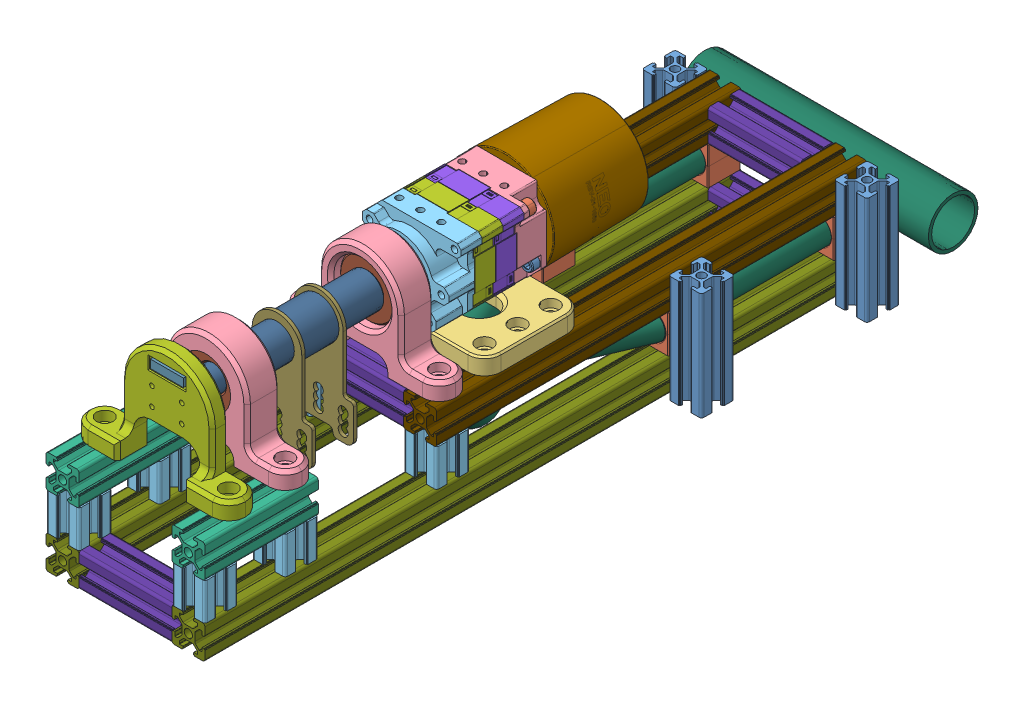
SolidWorks assembly SBW lower asm, configuration Default. Lengths in mm.
Overall size (150 145.03 440).
57 component instances, 26 part files, 180 mates.
Components (placement in the parent):
- MAXPlanetary 2-Stage-1: MAXPlanetary 2-Stage [Default] at origin size (89.61 89.51 122.08)
  - MAXPlanetary 2-Stage.STEP-1: MAXPlanetary 2-Stage.STEP [Default] at origin size (89.61 89.51 122.08)
    - REV-25-2109_2-Stage (No Shaft, For NEO).STEP-1: REV-25-2109_2-Stage (No Shaft, For NEO).STEP [Default] at origin size (65.15 54.03 73.34)
      - REV-25-2107_2-Stage.STEP-1: REV-25-2107_2-Stage.STEP [Default] at (0 0 6.35) x (-1 0 0) z (0 0 -1) size (65.15 54.03 73.34)
        - #10 Socket Head Cap Screws_0.500in Long.STEP-1: #10 Socket Head Cap Screws_0.500in Long.STEP [Default] at (21.1355 14.0872 12.7) x (0.923728 0.383049 0) z (0.383049 -0.923728 0) size (7.94 17.53 7.94)
        - #10 Socket Head Cap Screws_0.500in Long.STEP-2: #10 Socket Head Cap Screws_0.500in Long.STEP [Default] at (-21.1355 -14.0872 12.7) x (0.923728 0.383049 0) z (0.383049 -0.923728 0) size (7.94 17.53 7.94)
        - #10 Socket Head Cap Screws_1.500in Long.STEP-1: #10 Socket Head Cap Screws_1.500in Long.STEP [Default] at (-26.9919 21.4312 0) x (0.777574 0.628792 0) z (-0.628792 0.777574 0) size (7.94 42.93 7.94)
        - #10 Socket Head Cap Screws_1.500in Long.STEP-2: #10 Socket Head Cap Screws_1.500in Long.STEP [Default] at (26.9919 -21.4312 0) x (0.777574 0.628792 0) z (-0.628792 0.777574 0) size (7.94 42.93 7.94)
        - #10-32 Button Head Cap Screws_0.500in Long.STEP-1: #10-32 Button Head Cap Screws_0.500in Long.STEP [Default] at (0 0 -35.2425) x (0.655967 -0.754789 0) z (-0.754789 -0.655967 0) size (9.17 15.27 9.17)
      - REV-21-2106.STEP-1: REV-21-2106.STEP [Default] at origin size (61.91 50.8 19.05)
      - REV-21-2104.STEP-1: REV-21-2104.STEP [Default] at (0 0 44.45) x (0 0 1) z (-1 0 0) size (23.2 50.8 61.92)
      - REV-21-2108.STEP-1: REV-21-2108.STEP [Default] at (0 0 7.0985) x (-0.554615 -0.832107 0) z (0 0 -1) size (25.4 25.4 14.94)
    - REV-21-2101.STEP-1: REV-21-2101.STEP [Default] at (0 0 28.575) size (61.91 50.8 16.85)
    - REV-21-2102.STEP-1: REV-21-2102.STEP [Default] at (0 0 15.875) size (61.91 50.8 16.85)
    - REV-21-1650.STEP-1: REV-21-1650.STEP [Default] at (0 0 -9.525) x (0.554615 0.832107 0) z (0 0 1) size (64.41 64.76 93.26)
- shaft-1: shaft [Default] at (0 0 42.8625) x (0 0 1) z (-0.999764 0.021721 0) size (138 25 25)
- deep groove bearing 6202-1: deep groove bearing 6202 [默认] at (0 0 61.8625) size (35 35 11)
- shaft link-1: shaft link [默认] at (0 0 100.8625) size (42.5 73 2)
- shaft link-2: shaft link [默认] at (0 0 125.8625) size (42.5 73 2)
- AS5047P magnet-1: AS5047P magnet [Default] at (0 0 180.8625) x (1 0 0) z (0 1 0) size (6 2.5 6)
- deep groove bearing 6202-2: deep groove bearing 6202 [默认] at (0 0 155.8625) size (35 35 11)
- AS5047P-1: AS5047P [Default] at (0 6.4979 182.3625) size (22 28 12)
- frame asm-1: frame asm [默认] at (0 -66.9741 29.3625) x (0 0 1) z (0 1 0) size (330 260 46.82)
  - sw frame-1: sw frame [默认] at (-220 0 -0.0001) x (-1 0 0) z (0 0 -1) size (260.61 150 46.82)
  - middle frame-1: middle frame [默认] at (65 -130 -10) x (1 0 0) z (0 1 0) size (30 30 260) (hidden)
- T-slot frame long-1: T-slot frame long [默认] at (-37.9977 -88.1515 -180.6375) size (20 20 400)
- T-slot frame long-2: T-slot frame long [默认] at (37.9977 -88.1515 -180.6375) size (20 20 400)
- T-slot frame front-1: T-slot frame front [默认] at (27.9955 -88.1515 -170.6352) x (0 0 1) z (-1 0 0) size (20 20 56)
- T-slot frame upper-1: T-slot frame upper [默认] at (-37.9977 -45.7969 -180.6375) size (20 20 260)
- T-slot frame upper-2: T-slot frame upper [默认] at (37.9977 -45.7969 -180.6375) size (20 20 260)
- T-slot frame front-2: T-slot frame front [默认] at (27.9955 -45.7969 -170.6352) x (0 0 1) z (-1 0 0) size (20 20 56)
- T-slot frame side-1: T-slot frame side [默认] at (-58.0023 -35.7947 -170.6352) x (1 0 0) z (0 -1 0) size (20 20 65)
- T-slot frame side-2: T-slot frame side [默认] at (58.0023 -100.7947 -170.6352) x (0 0 -1) z (0 1 0) size (20 20 65)
- T-slot frame front-3: T-slot frame front [默认] at (28.0045 -45.7969 69.3602) x (0 0 1) z (-1 0 0) size (20 20 56)
- fitting-1: fitting [默认] at (38 -57.3867 -180.6375) size (20 11.18 20)
- fitting-2: fitting [默认] at (38 -76.5617 -180.6375) x (-1 0 0) z (0 0 1) size (20 11.18 20)
- fitting-3: fitting [默认] at (-38 -57.3867 -180.6375) size (20 11.18 20)
- fitting-4: fitting [默认] at (-38 -76.5617 -180.5051) x (-1 0 0) z (0 0 1) size (20 11.18 20)
- fitting-5: fitting [默认] at (-38 -57.3867 -80.6375) size (20 11.18 20)
- fitting-6: fitting [默认] at (-38 -76.5617 -80.6375) x (-1 0 0) z (0 0 1) size (20 11.18 20)
- fitting-7: fitting [默认] at (38 -57.3867 -80.6375) size (20 11.18 20)
- fitting-8: fitting [默认] at (38 -76.5617 -80.6375) x (-1 0 0) z (0 0 1) size (20 11.18 20)
- BLDC mount-1: BLDC mount [默认] at (0 -35.7947 20.475) x (1 0 0) z (0 1 0) size (96 60 10)
- front bearing mount-1: front bearing mount [默认] at (0 -35.5 67.8625) size (96 60.5 20)
- T-slot frame front-4: T-slot frame front [默认] at (28.0045 -88.1515 209.3602) x (0 0 1) z (-1 0 0) size (20 20 56)
- front bearing mount-2: front bearing mount [默认] at (0 -35.5 160.8625) x (-1 0 0) z (0 0 -1) size (96 60.5 20)
- T-slot frame side-9: T-slot frame side [默认] at (-58.0023 -35.7947 -70.6352) x (0 0 -1) z (0 -1 0) size (20 20 65)
- T-slot frame side-10: T-slot frame side [默认] at (58.0023 -35.7947 -70.6398) x (-1 0 0) z (0 -1 0) size (20 20 65)
- T-slot frame small-1: T-slot frame small [默认] at (-37.9977 -78.1492 69.3602) x (1 0 0) z (0 1 0) size (20 20 22.35)
- T-slot frame small-2: T-slot frame small [默认] at (37.9977 -55.7992 69.3602) x (1 0 0) z (0 -1 0) size (20 20 22.35)
- T-slot frame small-3: T-slot frame small [默认] at (37.9977 -78.1492 209.3602) x (1 0 0) z (0 1 0) size (20 20 22.35)
- T-slot frame small-4: T-slot frame small [默认] at (-37.9977 -55.7992 209.3602) x (1 0 0) z (0 -1 0) size (20 20 22.35)
- T-slot frame small-5: T-slot frame small [默认] at (-37.9977 -78.1492 160.8648) x (1 0 0) z (0 1 0) size (20 20 22.35)
- T-slot frame small-6: T-slot frame small [默认] at (37.9977 -55.7992 160.8602) x (1 0 0) z (0 -1 0) size (20 20 22.35)
- T-slot frame rear-1: T-slot frame rear [默认] at (-37.9977 -45.7969 150.8625) size (20 20 68.5)
- T-slot frame rear-2: T-slot frame rear [默认] at (37.9977 -45.7969 150.8625) size (20 20 68.5)
- lower AS5047P mount-2: lower AS5047P mount [Default] at (0 0 184.3625) x (0 0 1) z (-1 0 0) size (20 62.5 95)
Mates (geometry in assembly coordinates):
- front: coincident aligned: plane of MAXPlanetary 2-Stage-1 through (0 0 0) normal (0 0 1)
- top: coincident aligned: plane of MAXPlanetary 2-Stage-1 through (0 0 0) normal (0 1 0)
- right: coincident aligned: plane of MAXPlanetary 2-Stage-1 through (0 0 0) normal (1 0 0)
- 重合2: coincident anti-aligned: plane of MAXPlanetary 2-Stage-1/MAXPlanetary 2-Stage.STEP-1/REV-25-2109_2-Stage (No Shaft, For NEO).STEP-1/REV-21-2104.STEP-1 through (0 0 42.8625) normal (0 0 1); plane of shaft-1 through (0 0 42.8625) normal (0 0 -1)
- 同心1: concentric anti-aligned: circle of MAXPlanetary 2-Stage-1/MAXPlanetary 2-Stage.STEP-1/REV-25-2109_2-Stage (No Shaft, For NEO).STEP-1/REV-21-2104.STEP-1; cylinder of shaft-1 through (0 0 72.8625) axis (0 0 -1) radius 7.5
- 平行1: parallel anti-aligned: plane of MAXPlanetary 2-Stage-1/MAXPlanetary 2-Stage.STEP-1/REV-25-2109_2-Stage (No Shaft, For NEO).STEP-1/REV-21-2104.STEP-1 through (0.1594 7.3379 42.8625) normal (0.481071 -0.876682 0); plane of shaft-1 through (0.1593 7.3306 57.8625) normal (-0.481071 0.876682 0)
- 同心2: concentric aligned: cylinder of shaft-1 through (0 0 72.8625) axis (0 0 -1) radius 7.5; cylinder of deep groove bearing 6202-1 through (0 0 72.8625) axis (0 0 -1) radius 7.5
- 重合3: coincident anti-aligned: plane of shaft-1 through (0 0 72.8625) normal (0 0 -1); plane of deep groove bearing 6202-1 through (0 0 72.8625) normal (0 0 1)
- 同心3: concentric aligned: cylinder of shaft-1 through (0 0 102.8625) axis (0 0 -1) radius 10.5; cylinder of shaft link-1 through (0 0 102.8625) axis (0 0 -1) radius 10.5
- 重合4: coincident anti-aligned: plane of shaft-1 through (0 0 102.8625) normal (0 0 -1); plane of shaft link-1 through (-11.25 -55.5 102.8625) normal (0 0 1)
- 同心4: concentric aligned: cylinder of shaft-1 through (0 0 155.8625) axis (0 0 -1) radius 10.5; cylinder of shaft link-2 through (0 0 127.8625) axis (0 0 -1) radius 10.5
- 重合5: coincident anti-aligned: plane of shaft-1 through (0 0 125.8625) normal (0 0 1); plane of shaft link-2 through (-11.25 -55.5 125.8625) normal (0 0 -1)
- 重合6: coincident aligned: plane of shaft link-1 through (-15 0 102.8625) normal (-1 0 0); plane of shaft link-2 through (-15 0 127.8625) normal (-1 0 0)
- 重合7: coincident anti-aligned: plane of shaft-1 through (0 0 178.3625) normal (0 0 1); plane of AS5047P magnet-1 through (0 0 178.3625) normal (0 0 -1)
- 同心5: concentric aligned: cylinder of shaft-1 through (0 0 178.3625) axis (0 0 1) radius 3.5; cylinder of AS5047P magnet-1 through (0 0 178.3625) axis (0 0 1) radius 3
- 同心6: concentric aligned: cylinder of shaft-1 through (0 0 180.8625) axis (0 0 -1) radius 7.5; cylinder of deep groove bearing 6202-2 through (0 0 166.8625) axis (0 0 -1) radius 7.5
- 重合8: coincident anti-aligned: plane of shaft-1 through (0 0 155.8625) normal (0 0 1); plane of deep groove bearing 6202-2 through (0 0 155.8625) normal (0 0 -1)
- 距离1: distance = 1.5 mm anti-aligned: plane of AS5047P-1 through (0 6.4979 182.3625) normal (0 0 -1); plane of AS5047P magnet-1 through (0 0 180.8625) normal (0 0 1)
- 同心7: concentric: cylinder of AS5047P magnet-1 through (0 0 178.3625) axis (0 0 1) radius 3; point of AS5047P-1
- 平行4: parallel aligned: plane of MAXPlanetary 2-Stage-1/MAXPlanetary 2-Stage.STEP-1/REV-25-2109_2-Stage (No Shaft, For NEO).STEP-1/REV-21-2104.STEP-1 through (-30.1625 0 23.2597) normal (-1 0 0); plane of AS5047P-1 through (-11 20.4979 184.3625) normal (-1 0 0)
- 重合15: coincident anti-aligned: plane of AS5047P-1 through (0 6.4979 184.3625) normal (0 0 1); plane of lower AS5047P mount-1 through (0 0 184.3625) normal (0 0 -1)
- 同心8: concentric aligned: cylinder of AS5047P-1 through (-9 5.5 184.3625) axis (0 0 -1) radius 1.3; cylinder of lower AS5047P mount-1 through (-9 5.5 194.3625) axis (0 0 -1) radius 1.4
- 同心9: concentric aligned: cylinder of AS5047P-1 through (9 -5.5 184.3625) axis (0 0 -1) radius 1.3; cylinder of lower AS5047P mount-1 through (9 -5.5 194.3625) axis (0 0 -1) radius 1.4
- 同心10: concentric aligned: cylinder of shaft-1 through (0 0 72.8625) axis (0 0 -1) radius 7.5; cylinder of BLDC mount 1-1 through (0 0 58.975) axis (0 0 -1) radius 12.5
- 同心11: concentric anti-aligned: cylinder of MAXPlanetary 2-Stage-1/MAXPlanetary 2-Stage.STEP-1/REV-25-2109_2-Stage (No Shaft, For NEO).STEP-1/REV-21-2104.STEP-1 through (-17.9605 17.9605 53.975) axis (0 0 1) radius 2.0193; cylinder of BLDC mount 1-1 through (-17.96 17.96 58.975) axis (0 0 -1) radius 2
- 重合16: coincident anti-aligned: plane of MAXPlanetary 2-Stage-1/MAXPlanetary 2-Stage.STEP-1/REV-25-2109_2-Stage (No Shaft, For NEO).STEP-1/REV-21-2104.STEP-1 through (0 0 53.975) normal (0 0 1); plane of BLDC mount 1-1 through (0 0 53.975) normal (0 0 -1)
- 距离2: distance = 130 mm: plane of assembly through (0 0 0) normal (1 0 0); plane of assembly; plane of middle frame-1 through (130 -110.5456 57.9191) normal (1 0 0)
- 距离8: distance = 55 mm aligned: plane of sw frame-1 through (-75 -118.6918 -247.8837) normal (-1 0 0); plane of middle frame-1 through (-130 -110.5456 57.9191) normal (-1 0 0)
- 重合18: coincident anti-aligned: plane of sw frame-2 through (0 -92 -125.6375) normal (-1 0 0)
- 同心12: concentric anti-aligned: cylinder of sw frame-2 through (0 -107 94.3625) axis (0 1 0) radius 13
- 重合21: coincident: plane of sw frame-2 through (0 -77 94.3625) normal (0 1 0)
- 重合22: coincident aligned: plane of frame asm-1 through (0 -66.9741 29.3625) normal (1 0 0)
- 平行7: parallel aligned: plane of frame asm-1 through (0 -66.9741 29.3625) normal (0 0 1)
- 距离9: distance = 11.5 mm: plane of assembly; plane of frame asm-1; plane of shaft link-1 through (-11.25 -55.5 102.8625) normal (0 0 1)
- 相切1: tangent anti-aligned: cylinder of frame asm-1/sw frame-1 through (-38 -66.9742 -60.6375) axis (0 0 -1) radius 8; plane of 8875T911_Mount Plate for 1 4 -20 Thread Size-1 through (-58.6375 -58.9742 -180.6375) normal (0 -1 0)
- 平行8: parallel aligned: plane of 8875T911_Mount Plate for 1 4 -20 Thread Size-1 through (-58.6375 -56.5929 -180.6375) normal (0 1 0)
- 平行9: parallel anti-aligned: plane of 8875T911_Mount Plate for 1 4 -20 Thread Size-1 through (-17.3625 -56.5929 -180.6375) normal (0 0 -1)
- 同心14: concentric anti-aligned: cylinder of 8875T911_Mount Plate for 1 4 -20 Thread Size-1 through (-50.7 -56.5929 -171.1125) axis (0 -1 0) radius 3.175; cylinder of 8875T911_Mount Plate for 1 4 -20 Thread Size-2 through (-50.7 -36.5884 -171.1125) axis (0 1 0) radius 3.175
- 同心15: concentric anti-aligned: cylinder of 8875T911_Mount Plate for 1 4 -20 Thread Size-1 through (-25.3 -56.5929 -171.1125) axis (0 -1 0) radius 3.175; cylinder of 8875T911_Mount Plate for 1 4 -20 Thread Size-2 through (-25.3 -36.5884 -171.1125) axis (0 1 0) radius 3.175
- 重合25: coincident anti-aligned: plane of T-slot frame test-1 through (-38 -58.9742 89.3625) normal (0 -1 0); plane of 8875T911_Mount Plate for 1 4 -20 Thread Size-1 through (-58.6375 -56.5929 -180.6375) normal (0 1 0)
- 平行10: parallel aligned: cylinder of frame asm-1/sw frame-1 through (-38 -66.9742 -60.6375) axis (0 0 -1) radius 6; cylinder of T-slot frame test-1 through (-38 -48.9719 89.3625) axis (0 0 -1) radius 2.5
- 重合26: coincident anti-aligned: plane of T-slot frame test-1 through (-38 -38.9697 89.3625) normal (0 1 0); plane of 8875T911_Mount Plate for 1 4 -20 Thread Size-2 through (-17.3625 -36.5884 -180.6375) normal (0 -1 0)
- 距离11: distance = 10 mm anti-aligned: plane of T-slot frame test-1 through (-38 -48.9719 -180.6375) normal (0 0 -1); cylinder of frame asm-1/sw frame-1 through (75 -66.9742 -205.6375) axis (-1 0 0) radius 15
- 重合27: coincident aligned: plane of T-slot frame test-1 through (-38 -48.9719 -180.6375) normal (0 0 -1); plane of 8875T911_Mount Plate for 1 4 -20 Thread Size-2 through (-58.6375 -36.5884 -180.6375) normal (0 0 -1)
- 距离12: distance = 0 mm: plane of 8875T911_Mount Plate for 1 4 -20 Thread Size-2 through (-38 -34.2072 -171.1125) normal (-1 0 0); cylinder of T-slot frame test-1 through (-38 -48.9719 89.3625) axis (0 0 -1) radius 2.5
- 距离13: distance = 0 mm: plane of T-slot frame test-1 through (-38 -48.9719 -180.6375) normal (1 0 0); cylinder of frame asm-1/sw frame-1 through (-38 -66.9742 -60.6375) axis (0 0 -1) radius 8
- 重合28: coincident aligned: plane of 8875T911_Mount Plate for 1 4 -20 Thread Size-1 through (-58.6375 -56.5929 -161.5875) normal (-1 0 0); plane of 8875T911_Mount Plate for 1 4 -20 Thread Size-3 through (-58.6375 -58.9742 -79.6875) normal (-1 0 0)
- 重合29: coincident aligned: plane of 8875T911_Mount Plate for 1 4 -20 Thread Size-1 through (-58.6375 -56.5929 -180.6375) normal (0 1 0); plane of 8875T911_Mount Plate for 1 4 -20 Thread Size-3 through (-58.6375 -56.5929 -60.6375) normal (0 1 0)
- 重合30: coincident anti-aligned: circle of frame asm-1/sw frame-1; plane of 8875T911_Mount Plate for 1 4 -20 Thread Size-3 through (-17.3625 -58.9742 -60.6375) normal (0 0 1)
- 重合31: coincident aligned: plane of 8875T911_Mount Plate for 1 4 -20 Thread Size-2 through (-17.3625 -34.2072 -180.6375) normal (0 1 0); plane of 8875T911_Mount Plate for 1 4 -20 Thread Size-4 through (-17.3625 -34.2072 -79.6875) normal (0 1 0)
- 重合32: coincident aligned: plane of 8875T911_Mount Plate for 1 4 -20 Thread Size-3 through (-58.6375 -58.9742 -79.6875) normal (-1 0 0); plane of 8875T911_Mount Plate for 1 4 -20 Thread Size-4 through (-58.6375 -36.5884 -60.6375) normal (-1 0 0)
- 重合33: coincident aligned: plane of 8875T911_Mount Plate for 1 4 -20 Thread Size-3 through (-17.3625 -58.9742 -79.6875) normal (0 0 -1); plane of 8875T911_Mount Plate for 1 4 -20 Thread Size-4 through (-58.6375 -36.5884 -79.6875) normal (0 0 -1)
- 相切2: tangent aligned: cylinder of frame asm-1/sw frame-1 through (-38 -66.9742 -60.6375) axis (0 0 -1) radius 8; plane of 8875T914_Mount Plate for 3 8 -16 Thread Size-1 through (-9.425 -58.9742 -180.6375) normal (0 1 0)
- 重合34: coincident aligned: plane of T-slot frame test-1 through (-38 -48.9719 -180.6375) normal (0 0 -1); plane of 8875T914_Mount Plate for 3 8 -16 Thread Size-1 through (-66.575 -62.1492 -180.6375) normal (0 0 -1)
- 距离14: distance = 0 mm: plane of 8875T914_Mount Plate for 3 8 -16 Thread Size-1 through (-38 -58.9742 -167.9375) normal (-1 0 0); cylinder of frame asm-1/sw frame-1 through (-38 -66.9742 -60.6375) axis (0 0 -1) radius 8
- 平行11: parallel aligned: plane of 8875T914_Mount Plate for 3 8 -16 Thread Size-1 through (-9.425 -58.9742 -180.6375) normal (0 1 0)
- 重合36: coincident anti-aligned: plane of T-slot frame test-1 through (-38 -58.9742 89.3625) normal (0 -1 0); plane of 8875T914_Mount Plate for 3 8 -16 Thread Size-1 through (-9.425 -58.9742 -180.6375) normal (0 1 0)
- 同心16: concentric aligned: cylinder of 8875T914_Mount Plate for 3 8 -16 Thread Size-1 through (-20.5375 -62.1492 -167.9375) axis (0 1 0) radius 4.7625; cylinder of U-shape bolt-1 through (-20.5375 -70.2447 -167.9375) axis (0 1 0) radius 4.7625
- 同心17: concentric aligned: cylinder of 8875T914_Mount Plate for 3 8 -16 Thread Size-1 through (-55.4625 -62.1492 -167.9375) axis (0 1 0) radius 4.7625; cylinder of U-shape bolt-1 through (-55.4625 -57.5447 -167.9375) axis (0 1 0) radius 4.7625
- 重合37: coincident anti-aligned: plane of T-slot frame test-1 through (-38 -38.9697 89.3625) normal (0 1 0); plane of 8875T914_Mount Plate for 3 8 -16 Thread Size-2 through (-66.575 -38.9697 -180.6375) normal (0 -1 0)
- 重合38: coincident aligned: plane of 8875T914_Mount Plate for 3 8 -16 Thread Size-1 through (-66.575 -62.1492 -180.6375) normal (0 0 -1); plane of 8875T914_Mount Plate for 3 8 -16 Thread Size-2 through (-9.425 -35.7947 -180.6375) normal (0 0 -1)
- 重合39: coincident aligned: plane of 8875T914_Mount Plate for 3 8 -16 Thread Size-1 through (-66.575 -62.1492 -155.2375) normal (-1 0 0); plane of 8875T914_Mount Plate for 3 8 -16 Thread Size-2 through (-66.575 -35.7947 -155.2375) normal (-1 0 0)
- 距离15: distance = 10 mm aligned: plane of U-shape bolt-1 through (-20.5375 -25.7947 -167.9375) normal (0 1 0); plane of 8875T914_Mount Plate for 3 8 -16 Thread Size-2 through (-66.575 -35.7947 -180.6375) normal (0 1 0)
- 同心18: concentric: cylinder of shaft link-2 through (0 -46.9741 127.8625) axis (0 0 -1) radius 3
- 距离16: distance = 10 mm anti-aligned: plane of T-slot frame long-1 through (-37.9977 -88.1515 -180.6375) normal (0 0 -1); cylinder of frame asm-1/sw frame-1 through (75 -66.9742 -205.6375) axis (-1 0 0) radius 15
- 平行12: parallel aligned: cylinder of frame asm-1/sw frame-1 through (-38 -66.9742 -60.6375) axis (0 0 -1) radius 6; cylinder of T-slot frame long-1 through (-37.9977 -88.1515 219.3625) axis (0 0 -1) radius 2.5
- 重合41: coincident aligned: plane of T-slot frame long-1 through (-37.9977 -88.1515 -180.6375) normal (0 0 -1); plane of T-slot frame long-2 through (37.9977 -88.1515 -180.6375) normal (0 0 -1)
- 平行13: parallel aligned: cylinder of frame asm-1/sw frame-1 through (38 -66.9742 -60.6375) axis (0 0 -1) radius 6; cylinder of T-slot frame long-2 through (37.9977 -88.1515 219.3625) axis (0 0 -1) radius 2.5
- 平行14: parallel anti-aligned: plane of T-slot frame long-1 through (-48 -88.1515 219.3625) normal (-1 0 0)
- 平行15: parallel anti-aligned: plane of T-slot frame long-1 through (-37.9977 -98.1537 219.3625) normal (0 -1 0)
- 距离17: distance = 2 mm aligned: plane of T-slot frame long-1 through (-48 -88.1515 219.3625) normal (-1 0 0); cylinder of frame asm-1/sw frame-1 through (-38 -66.9742 -60.6375) axis (0 0 -1) radius 8
- 距离18: distance = 3.175 mm anti-aligned: plane of T-slot frame long-1 through (-37.9977 -78.1492 219.3625) normal (0 1 0); cylinder of frame asm-1/sw frame-1 through (-38 -66.9742 -60.6375) axis (0 0 -1) radius 8
- 平行16: parallel aligned: plane of T-slot frame long-2 through (37.9977 -78.1492 219.3625) normal (0 1 0)
- 平行17: parallel aligned: plane of frame asm-1 through (0 -66.9741 29.3625) normal (0 1 0); plane of T-slot frame long-2 through (37.9977 -78.1492 219.3625) normal (0 1 0)
- 距离21: distance = 2 mm aligned: plane of T-slot frame long-2 through (48 -88.1515 219.3625) normal (1 0 0); cylinder of frame asm-1/sw frame-1 through (38 -66.9742 -60.6375) axis (0 0 -1) radius 8
- 距离22: distance = 3.175 mm anti-aligned: plane of T-slot frame long-2 through (37.9977 -78.1492 219.3625) normal (0 1 0); cylinder of frame asm-1/sw frame-1 through (38 -66.9742 -60.6375) axis (0 0 -1) radius 8
- 重合46: coincident aligned: plane of T-slot frame long-2 through (37.9977 -98.1537 219.3625) normal (0 -1 0); plane of T-slot frame front-1 through (-28.0045 -98.1537 -170.6352) normal (0 -1 0)
- 重合47: coincident anti-aligned: plane of T-slot frame long-2 through (27.9955 -88.1515 219.3625) normal (-1 0 0); plane of T-slot frame front-1 through (27.9955 -88.1515 -170.6352) normal (1 0 0)
- 重合48: coincident aligned: plane of T-slot frame long-2 through (37.9977 -88.1515 -180.6375) normal (0 0 -1); plane of T-slot frame front-1 through (-28.0045 -88.1515 -180.6375) normal (0 0 -1)
- 重合49: coincident aligned: plane of T-slot frame long-1 through (-37.9977 -88.1515 -180.6375) normal (0 0 -1); plane of T-slot frame upper-1 through (-37.9977 -45.7969 -180.6375) normal (0 0 -1)
- 距离23: distance = 3.175 mm anti-aligned: plane of T-slot frame upper-1 through (-37.9977 -55.7992 79.3625) normal (0 -1 0); cylinder of frame asm-1/sw frame-1 through (-38 -66.9742 -60.6375) axis (0 0 -1) radius 8
- 重合50: coincident aligned: plane of T-slot frame long-1 through (-48 -88.1515 219.3625) normal (-1 0 0); plane of T-slot frame upper-1 through (-48 -45.7969 79.3625) normal (-1 0 0)
- 重合51: coincident aligned: plane of T-slot frame long-2 through (37.9977 -88.1515 -180.6375) normal (0 0 -1); plane of T-slot frame upper-2 through (37.9977 -45.7969 -180.6375) normal (0 0 -1)
- 重合52: coincident aligned: plane of T-slot frame upper-1 through (-37.9977 -35.7947 79.3625) normal (0 1 0); plane of T-slot frame upper-2 through (37.9977 -35.7947 79.3625) normal (0 1 0)
- 重合53: coincident aligned: plane of T-slot frame long-2 through (48 -88.1515 219.3625) normal (1 0 0); plane of T-slot frame upper-2 through (48 -45.7969 79.3625) normal (1 0 0)
- 重合54: coincident anti-aligned: plane of T-slot frame upper-2 through (27.9955 -45.7969 79.3625) normal (-1 0 0); plane of T-slot frame front-2 through (27.9955 -45.7969 -170.6352) normal (1 0 0)
- 重合55: coincident aligned: plane of T-slot frame upper-2 through (37.9977 -45.7969 -180.6375) normal (0 0 -1); plane of T-slot frame front-2 through (-28.0045 -45.7969 -180.6375) normal (0 0 -1)
- 重合56: coincident aligned: plane of T-slot frame upper-2 through (37.9977 -35.7947 79.3625) normal (0 1 0); plane of T-slot frame front-2 through (-28.0045 -35.7947 -170.6352) normal (0 1 0)
- 重合57: coincident anti-aligned: plane of T-slot frame upper-1 through (-48 -45.7969 79.3625) normal (-1 0 0); plane of T-slot frame side-1 through (-48 -100.7947 -170.6352) normal (1 0 0)
- 重合58: coincident aligned: plane of T-slot frame upper-1 through (-37.9977 -35.7947 79.3625) normal (0 1 0); plane of T-slot frame side-1 through (-58.0023 -35.7947 -170.6352) normal (0 1 0)
- 重合59: coincident aligned: plane of T-slot frame upper-1 through (-37.9977 -45.7969 -180.6375) normal (0 0 -1); plane of T-slot frame side-1 through (-58.0023 -100.7947 -180.6375) normal (0 0 -1)
- 重合60: coincident anti-aligned: plane of T-slot frame long-2 through (48 -88.1515 219.3625) normal (1 0 0); plane of T-slot frame side-2 through (48 -35.7947 -170.6352) normal (-1 0 0)
- 重合61: coincident aligned: plane of T-slot frame upper-2 through (37.9977 -45.7969 -180.6375) normal (0 0 -1); plane of T-slot frame side-2 through (58.0023 -35.7947 -180.6375) normal (0 0 -1)
- 重合62: coincident aligned: plane of T-slot frame upper-2 through (37.9977 -35.7947 79.3625) normal (0 1 0); plane of T-slot frame side-2 through (58.0023 -35.7947 -170.6352) normal (0 1 0)
- 重合63: coincident aligned: plane of T-slot frame upper-1 through (-37.9977 -35.7947 79.3625) normal (0 1 0); plane of T-slot frame side-3 through (-58.0023 -35.7947 69.3602) normal (0 1 0)
- 重合64: coincident anti-aligned: plane of T-slot frame long-1 through (-48 -88.1515 219.3625) normal (-1 0 0); plane of T-slot frame side-3 through (-48 -35.7947 69.3602) normal (1 0 0)
- 重合65: coincident aligned: plane of T-slot frame upper-1 through (-37.9977 -45.7969 79.3625) normal (0 0 1); plane of T-slot frame side-3 through (-58.0023 -35.7947 79.3625) normal (0 0 1)
- 重合66: coincident aligned: plane of T-slot frame upper-2 through (37.9977 -35.7947 79.3625) normal (0 1 0); plane of T-slot frame side-4 through (58.0023 -35.7947 69.3602) normal (0 1 0)
- 重合67: coincident anti-aligned: plane of T-slot frame upper-2 through (48 -45.7969 79.3625) normal (1 0 0); plane of T-slot frame side-4 through (48 -100.7947 69.3602) normal (-1 0 0)
- 重合68: coincident aligned: plane of T-slot frame upper-2 through (37.9977 -45.7969 79.3625) normal (0 0 1); plane of T-slot frame side-4 through (58.0023 -100.7947 79.3625) normal (0 0 1)
- 重合69: coincident anti-aligned: plane of T-slot frame upper-1 through (-27.9955 -45.7969 79.3625) normal (1 0 0); plane of T-slot frame front-3 through (-27.9955 -45.7969 69.3602) normal (-1 0 0)
- 重合70: coincident aligned: plane of T-slot frame upper-2 through (37.9977 -35.7947 79.3625) normal (0 1 0); plane of T-slot frame front-3 through (-27.9955 -35.7947 69.3602) normal (0 1 0)
- 重合71: coincident aligned: plane of T-slot frame upper-2 through (37.9977 -45.7969 79.3625) normal (0 0 1); plane of T-slot frame front-3 through (-27.9955 -45.7969 79.3625) normal (0 0 1)
- 重合72: coincident anti-aligned: plane of T-slot frame upper-2 through (37.9977 -55.7992 79.3625) normal (0 -1 0); plane of fitting-1 through (28 -55.7992 -160.6375) normal (0 1 0)
- 重合73: coincident aligned: plane of T-slot frame upper-2 through (48 -45.7969 79.3625) normal (1 0 0); plane of fitting-1 through (48 -55.7992 -160.6375) normal (1 0 0)
- 重合75: coincident aligned: plane of T-slot frame upper-2 through (37.9977 -45.7969 -180.6375) normal (0 0 -1); plane of fitting-1 through (38 -66.9742 -180.6375) normal (0 0 -1)
- 重合76: coincident anti-aligned: plane of T-slot frame long-2 through (37.9977 -78.1492 219.3625) normal (0 1 0); plane of fitting-2 through (48 -78.1492 -160.6375) normal (0 -1 0)
- 重合77: coincident aligned: plane of fitting-1 through (38 -66.9742 -180.6375) normal (0 0 -1); plane of fitting-2 through (38 -66.9742 -180.6375) normal (0 0 -1)
- 重合78: coincident aligned: plane of T-slot frame upper-1 through (-37.9977 -45.7969 -180.6375) normal (0 0 -1); plane of fitting-3 through (-38 -66.9742 -180.6375) normal (0 0 -1)
- 重合79: coincident aligned: plane of T-slot frame upper-1 through (-48 -45.7969 79.3625) normal (-1 0 0); plane of fitting-3 through (-48 -58.9742 -160.6375) normal (-1 0 0)
- 重合80: coincident anti-aligned: plane of T-slot frame long-1 through (-37.9977 -78.1492 219.3625) normal (0 1 0); plane of fitting-4 through (-28 -78.1492 -160.5051) normal (0 -1 0)
- 重合81: coincident aligned: plane of fitting-3 through (-48 -58.9742 -160.6375) normal (-1 0 0); plane of fitting-4 through (-48 -78.1492 -160.5051) normal (-1 0 0)
- 重合82: coincident anti-aligned: plane of T-slot frame upper-1 through (-37.9977 -55.7992 79.3625) normal (0 -1 0); plane of fitting-5 through (-48 -55.7992 -60.6375) normal (0 1 0)
- 重合83: coincident aligned: plane of T-slot frame upper-1 through (-48 -45.7969 79.3625) normal (-1 0 0); plane of fitting-5 through (-48 -58.9742 -60.6375) normal (-1 0 0)
- 重合87: coincident aligned: plane of fitting-5 through (-38 -66.9742 -60.6375) normal (0 0 1); plane of fitting-6 through (-38 -66.9742 -60.6375) normal (0 0 1)
- 重合88: coincident aligned: plane of fitting-5 through (-48 -58.9742 -60.6375) normal (-1 0 0); plane of fitting-6 through (-48 -78.1492 -60.6375) normal (-1 0 0)
- 重合89: coincident anti-aligned: plane of T-slot frame long-1 through (-37.9977 -78.1492 219.3625) normal (0 1 0); plane of fitting-6 through (-28 -78.1492 -60.6375) normal (0 -1 0)
- 重合90: coincident anti-aligned: plane of T-slot frame upper-2 through (37.9977 -55.7992 79.3625) normal (0 -1 0); plane of fitting-7 through (28 -55.7992 -60.6375) normal (0 1 0)
- 重合91: coincident aligned: plane of T-slot frame upper-2 through (48 -45.7969 79.3625) normal (1 0 0); plane of fitting-7 through (48 -55.7992 -60.6375) normal (1 0 0)
- 重合92: coincident anti-aligned: circle of frame asm-1/sw frame-1; plane of fitting-7 through (38 -66.9742 -60.6375) normal (0 0 1)
- 重合93: coincident aligned: plane of fitting-7 through (28 -58.9742 -60.6375) normal (-1 0 0); plane of fitting-8 through (28 -78.1492 -60.6375) normal (-1 0 0)
- 重合94: coincident aligned: plane of fitting-7 through (38 -66.9742 -80.6375) normal (0 0 -1); plane of fitting-8 through (38 -66.9742 -80.6375) normal (0 0 -1)
- 重合96: coincident anti-aligned: plane of T-slot frame long-2 through (37.9977 -78.1492 219.3625) normal (0 1 0); plane of fitting-8 through (48 -78.1492 -60.6375) normal (0 -1 0)
- 重合97: coincident anti-aligned: plane of T-slot frame upper-1 through (-37.9977 -35.7947 79.3625) normal (0 1 0); plane of BLDC mount-1 through (0 -35.7947 20.475) normal (0 -1 0)
- 重合98: coincident aligned: plane of T-slot frame upper-1 through (-48 -45.7969 79.3625) normal (-1 0 0); plane of BLDC mount-1 through (-48 -25.7947 -9.525) normal (-1 0 0)
- 重合99: coincident anti-aligned: plane of MAXPlanetary 2-Stage-1/MAXPlanetary 2-Stage.STEP-1/REV-21-1650.STEP-1 through (0 0 -9.525) normal (0 0 1); plane of BLDC mount-1 through (-48 -25.7947 -9.525) normal (0 0 -1)
- 平行22: parallel anti-aligned: plane of T-slot frame upper-1 through (-37.9977 -35.7947 79.3625) normal (0 1 0); plane of front bearing mount-1 through (0 -35.5 67.8625) normal (0 -1 0)
- 重合102: coincident anti-aligned: plane of deep groove bearing 6202-1 through (0 0 61.8625) normal (0 0 -1); plane of front bearing mount-1 through (0 0 61.8625) normal (0 0 1)
- 同心25: concentric anti-aligned: cylinder of deep groove bearing 6202-1 through (0 0 72.8625) axis (0 0 -1) radius 17.5; cylinder of front bearing mount-1 through (0 0 61.8625) axis (0 0 1) radius 17.6
- 重合106: coincident aligned: plane of T-slot frame long-1 through (-37.9977 -98.1537 219.3625) normal (0 -1 0); plane of T-slot frame front-4 through (-27.9955 -98.1537 209.3602) normal (0 -1 0)
- 重合107: coincident aligned: plane of T-slot frame long-1 through (-37.9977 -88.1515 219.3625) normal (0 0 1); plane of T-slot frame front-4 through (-27.9955 -88.1515 219.3625) normal (0 0 1)
- 重合108: coincident anti-aligned: plane of T-slot frame long-1 through (-27.9955 -88.1515 219.3625) normal (1 0 0); plane of T-slot frame front-4 through (-27.9955 -88.1515 209.3602) normal (-1 0 0)
- 重合109: coincident aligned: plane of T-slot frame long-1 through (-37.9977 -98.1537 219.3625) normal (0 -1 0); plane of T-slot frame side-5 through (-58.0023 -98.1537 209.3602) normal (0 -1 0)
- 重合110: coincident anti-aligned: plane of T-slot frame long-1 through (-48 -88.1515 219.3625) normal (-1 0 0); plane of T-slot frame side-5 through (-48 -98.1537 209.3602) normal (1 0 0)
- 重合111: coincident aligned: plane of T-slot frame long-1 through (-37.9977 -88.1515 219.3625) normal (0 0 1); plane of T-slot frame side-5 through (-58.0023 -98.1537 219.3625) normal (0 0 1)
- 重合112: coincident aligned: plane of T-slot frame long-2 through (37.9977 -98.1537 219.3625) normal (0 -1 0); plane of T-slot frame side-6 through (58.0023 -98.1537 209.3602) normal (0 -1 0)
- 重合113: coincident anti-aligned: plane of T-slot frame long-2 through (48 -88.1515 219.3625) normal (1 0 0); plane of T-slot frame side-6 through (48 -98.1537 209.3602) normal (-1 0 0)
- 重合114: coincident aligned: plane of T-slot frame long-2 through (37.9977 -88.1515 219.3625) normal (0 0 1); plane of T-slot frame side-6 through (58.0023 -98.1537 219.3625) normal (0 0 1)
- 重合115: coincident: plane of T-slot frame long-2 through (37.9977 -98.1537 219.3625) normal (0 -1 0); plane of T-slot frame side-7 through (44.8435 -93.1903 162.7165) normal (0 -1 0)
- 重合116: coincident: plane of T-slot frame long-2 through (48 -88.1515 219.3625) normal (1 0 0); plane of T-slot frame side-7 through (34.8412 -93.1903 162.7165) normal (-1 0 0)
- 重合117: coincident: plane of T-slot frame long-1 through (-48 -88.1515 219.3625) normal (-1 0 0); plane of T-slot frame side-8 through (-37.7941 -92.04 162.8017) normal (1 0 0)
- 重合118: coincident: plane of T-slot frame side-5 through (-58.0023 -98.1537 209.3602) normal (0 -1 0); plane of T-slot frame side-8 through (-47.7963 -92.04 162.8017) normal (0 -1 0)
- 同心26: concentric aligned: cylinder of deep groove bearing 6202-2 through (0 0 166.8625) axis (0 0 -1) radius 17.5; cylinder of front bearing mount-2 through (0 0 166.8625) axis (0 0 -1) radius 17.6
- 重合119: coincident anti-aligned: plane of deep groove bearing 6202-2 through (0 0 166.8625) normal (0 0 1); plane of front bearing mount-2 through (0 0 166.8625) normal (0 0 -1)
- 重合120: coincident aligned: plane of front bearing mount-1 through (0 -35.5 67.8625) normal (0 -1 0); plane of front bearing mount-2 through (0 -35.5 160.8625) normal (0 -1 0)
- 重合121: coincident aligned: plane of T-slot frame side-8 through (-58.0023 -98.1537 150.8625) normal (0 0 -1); plane of front bearing mount-2 through (48 -25.5 150.8625) normal (0 0 -1)
- 重合122: coincident aligned: plane of T-slot frame side-7 through (58.0023 -98.1537 150.8625) normal (0 0 -1); plane of front bearing mount-2 through (48 -25.5 150.8625) normal (0 0 -1)
- 重合123: coincident aligned: plane of T-slot frame upper-1 through (-37.9977 -35.7947 79.3625) normal (0 1 0); plane of T-slot frame side-9 through (-58.0023 -35.7947 -70.6352) normal (0 1 0)
- 重合124: coincident anti-aligned: plane of T-slot frame upper-1 through (-48 -45.7969 79.3625) normal (-1 0 0); plane of T-slot frame side-9 through (-48 -100.7947 -70.6352) normal (1 0 0)
- 重合125: coincident aligned: plane of fitting-5 through (-38 -66.9742 -80.6375) normal (0 0 -1); plane of T-slot frame side-9 through (-58.0023 -100.7947 -80.6375) normal (0 0 -1)
- 重合126: coincident aligned: plane of T-slot frame upper-2 through (37.9977 -35.7947 79.3625) normal (0 1 0); plane of T-slot frame side-10 through (58.0023 -35.7947 -70.6398) normal (0 1 0)
- 重合127: coincident anti-aligned: plane of T-slot frame upper-2 through (48 -45.7969 79.3625) normal (1 0 0); plane of T-slot frame side-10 through (48 -100.7947 -70.6398) normal (-1 0 0)
- 重合128: coincident aligned: plane of fitting-7 through (38 -66.9742 -60.6375) normal (0 0 1); plane of T-slot frame side-10 through (58.0023 -100.7947 -60.6375) normal (0 0 1)
- 重合129: coincident anti-aligned: plane of T-slot frame upper-1 through (-37.9977 -55.7992 79.3625) normal (0 -1 0); plane of T-slot frame small-1 through (-37.9977 -55.7992 69.3602) normal (0 1 0)
- 重合130: coincident aligned: plane of T-slot frame upper-1 through (-37.9977 -45.7969 79.3625) normal (0 0 1); plane of T-slot frame small-1 through (-37.9977 -55.7992 79.3625) normal (0 0 1)
- 重合131: coincident aligned: plane of T-slot frame long-1 through (-48 -88.1515 219.3625) normal (-1 0 0); plane of T-slot frame small-1 through (-48 -55.7992 69.3602) normal (-1 0 0)
- 重合132: coincident anti-aligned: plane of T-slot frame long-2 through (37.9977 -78.1492 219.3625) normal (0 1 0); plane of T-slot frame small-2 through (37.9977 -78.1492 69.3602) normal (0 -1 0)
- 重合133: coincident aligned: plane of T-slot frame upper-2 through (37.9977 -45.7969 79.3625) normal (0 0 1); plane of T-slot frame small-2 through (37.9977 -78.1492 79.3625) normal (0 0 1)
- 重合134: coincident aligned: plane of T-slot frame upper-2 through (48 -45.7969 79.3625) normal (1 0 0); plane of T-slot frame small-2 through (48 -78.1492 69.3602) normal (1 0 0)
- 重合135: coincident anti-aligned: plane of T-slot frame long-2 through (37.9977 -78.1492 219.3625) normal (0 1 0); plane of T-slot frame small-3 through (37.9977 -78.1492 209.3602) normal (0 -1 0)
- 重合136: coincident aligned: plane of T-slot frame long-2 through (48 -88.1515 219.3625) normal (1 0 0); plane of T-slot frame small-3 through (48 -55.7992 209.3602) normal (1 0 0)
- 重合137: coincident aligned: plane of T-slot frame front-4 through (-27.9955 -88.1515 219.3625) normal (0 0 1); plane of T-slot frame small-3 through (37.9977 -55.7992 219.3625) normal (0 0 1)
- 重合138: coincident anti-aligned: plane of T-slot frame long-1 through (-37.9977 -78.1492 219.3625) normal (0 1 0); plane of T-slot frame small-4 through (-37.9977 -78.1492 209.3602) normal (0 -1 0)
- 重合139: coincident aligned: plane of T-slot frame front-4 through (-27.9955 -88.1515 219.3625) normal (0 0 1); plane of T-slot frame small-4 through (-37.9977 -78.1492 219.3625) normal (0 0 1)
- 重合140: coincident aligned: plane of T-slot frame long-1 through (-48 -88.1515 219.3625) normal (-1 0 0); plane of T-slot frame small-4 through (-48 -78.1492 209.3602) normal (-1 0 0)
- 重合141: coincident anti-aligned: plane of T-slot frame long-1 through (-37.9977 -78.1492 219.3625) normal (0 1 0); plane of T-slot frame small-5 through (-37.9977 -78.1492 160.8648) normal (0 -1 0)
- 重合142: coincident aligned: plane of front bearing mount-2 through (48 -25.5 150.8625) normal (0 0 -1); plane of T-slot frame small-5 through (-37.9977 -55.7992 150.8625) normal (0 0 -1)
- 重合143: coincident aligned: plane of T-slot frame long-1 through (-48 -88.1515 219.3625) normal (-1 0 0); plane of T-slot frame small-5 through (-48 -55.7992 160.8648) normal (-1 0 0)
- 重合144: coincident anti-aligned: plane of T-slot frame long-2 through (37.9977 -78.1492 219.3625) normal (0 1 0); plane of T-slot frame small-6 through (37.9977 -78.1492 160.8602) normal (0 -1 0)
- 重合145: coincident aligned: plane of front bearing mount-2 through (48 -25.5 170.8625) normal (0 0 1); plane of T-slot frame small-6 through (37.9977 -78.1492 170.8625) normal (0 0 1)
- 重合146: coincident aligned: plane of T-slot frame long-2 through (27.9955 -88.1515 219.3625) normal (-1 0 0); plane of T-slot frame small-6 through (27.9955 -78.1492 160.8602) normal (-1 0 0)
- 重合147: coincident aligned: plane of T-slot frame small-5 through (-37.9977 -55.7992 150.8625) normal (0 0 -1); plane of T-slot frame rear-1 through (-37.9977 -45.7969 150.8625) normal (0 0 -1)
- 重合148: coincident anti-aligned: plane of T-slot frame small-5 through (-37.9977 -55.7992 160.8648) normal (0 1 0); plane of T-slot frame rear-1 through (-37.9977 -55.7992 219.3625) normal (0 -1 0)
- 重合149: coincident aligned: plane of T-slot frame small-5 through (-48 -55.7992 160.8648) normal (-1 0 0); plane of T-slot frame rear-1 through (-48 -45.7969 219.3625) normal (-1 0 0)
- 重合150: coincident aligned: plane of T-slot frame small-3 through (37.9977 -55.7992 219.3625) normal (0 0 1); plane of T-slot frame rear-2 through (37.9977 -45.7969 219.3625) normal (0 0 1)
- 重合151: coincident anti-aligned: plane of T-slot frame small-3 through (37.9977 -55.7992 209.3602) normal (0 1 0); plane of T-slot frame rear-2 through (37.9977 -55.7992 219.3625) normal (0 -1 0)
- 重合152: coincident aligned: plane of T-slot frame small-3 through (27.9955 -55.7992 209.3602) normal (-1 0 0); plane of T-slot frame rear-2 through (27.9955 -45.7969 219.3625) normal (-1 0 0)
- 同心29: concentric: cylinder of AS5047P-1 through (-9 5.5 184.3625) axis (0 0 -1) radius 1.3; cylinder of lower AS5047P mount-2 through (-9 5.5 174.3625) axis (0 0 1) radius 1.4
- 同心30: concentric: cylinder of AS5047P-1 through (-9 -5.5 184.3625) axis (0 0 -1) radius 1.3; cylinder of lower AS5047P mount-2 through (-9 -5.5 174.3625) axis (0 0 1) radius 1.4
- 重合155: coincident anti-aligned: plane of AS5047P-1 through (0 6.4979 184.3625) normal (0 0 1); plane of lower AS5047P mount-2 through (0 0 184.3625) normal (0 0 -1)
